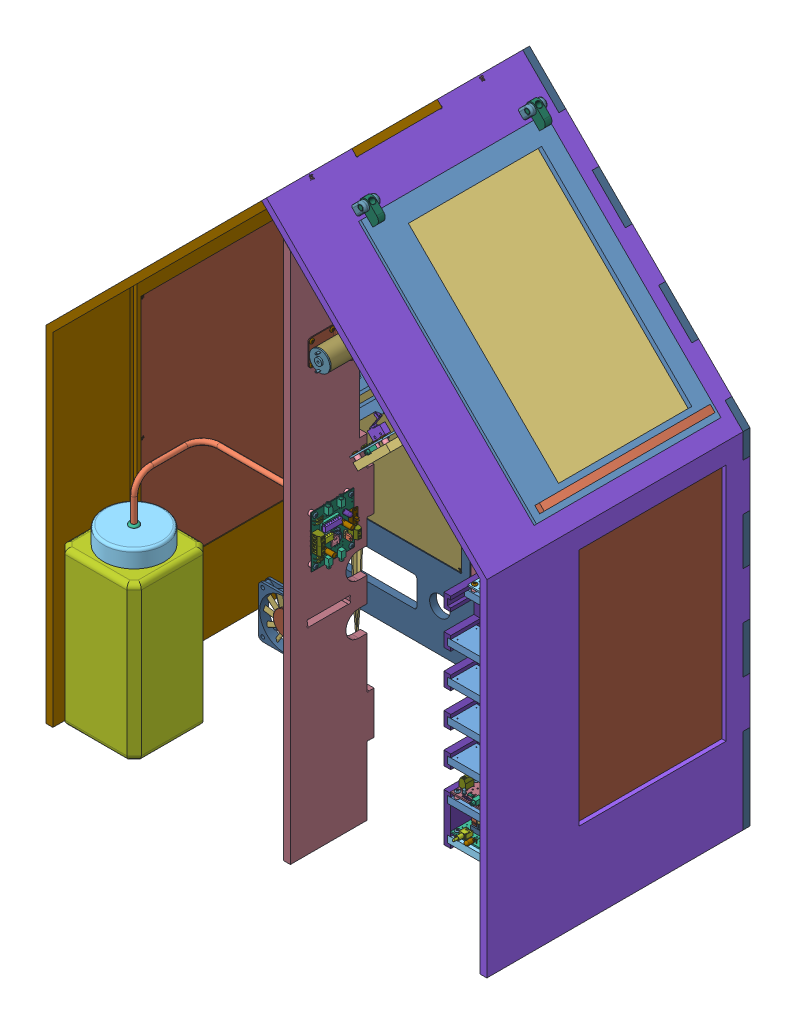
SolidWorks assembly Serre de base VDS, configuration guillotine. Lengths in mm.
Overall size (183.35 183.35 75.13).
351 component instances, 97 part files, 150 mates.
Components (placement in the parent):
- FONDINTERIEUR-1: FONDINTERIEUR [Défaut] at (-62.876 -300.5478 -4) (hidden)
- Crémallière M3-3-1: Crémallière M3-3 [Défaut] at (-39.5374 94.1308 4) x (0.707107 0.707107 0) z (0 0 1)
- Rondelle métal 3 x 12-1: Rondelle métal 3 x 12 [Défaut] at (57.939 191.6778 8)
- VIs TC 3 x 13-1: VIs TC 3 x 13 [Défaut] at (57.939 191.6778 2.4) x (1 0 0) z (0 -1 0) (hidden)
- VIs TC 3 x 13-2: VIs TC 3 x 13 [Défaut] at (22.5836 156.3225 2.4) x (1 0 0) z (0 -1 0) (hidden)
- Rondelle métal 3 x 12-2: Rondelle métal 3 x 12 [Défaut] at (22.5836 156.3225 8)
- Prépa 06 module Microrupteur-1: Prépa 06 module Microrupteur [Défaut] at (80.8247 148.8026 12.3834) x (0.707107 0.707107 0) z (-0.707107 0.707107 0) size (54 40.91 35.34)
  - support capteur-1: support capteur [Défaut] at (85.4284 22.7312 -4) size (54 38 8)
  - Entretoise CI-1: Entretoise CI [Défaut] at (-25.3985 -17.6166 4) size (5.9 5.9 4.1)
  - Entretoise CI-2: Entretoise CI [Défaut] at (-25.3985 4.3834 4) size (5.9 5.9 4.1)
  - Entretoise CI-3: Entretoise CI [Défaut] at (20.6015 -17.6166 4) size (5.9 5.9 4.1)
  - Entretoise CI-4: Entretoise CI [Défaut] at (20.6015 4.3834 4) size (5.9 5.9 4.1)
  - Module Microrupteur K-AP-MMR-1: Module Microrupteur K-AP-MMR [Défaut] at (24.602 -8.2581 10.6485) x (0 1 0) z (1 0 0) size (32.91 28.24 54)
    - CI-AP-MLBP avec jack-1: CI-AP-MLBP avec jack [Défaut] at (1.5279 -1.3102 0) size (32.91 8.01 54)
      - CI BP et DEL-1: CI BP et DEL [Défaut] at (-14.8869 -1.2382 0) size (30 1.6 54)
      - Embase jack 2.5-1: Embase jack 2.5 [Défaut] at (-14.8868 -1.2382 -27.0002) x (1 0 0) z (0 0 -1) size (10.81 8.01 5)
    - Résistance 10 K pas 11-1: Résistance 10 K pas 11 [Défaut] at (-6.8591 0.4515 -37.4997) x (0 0 -1) z (1 0 0) size (11.5 4.15 2.3)
    - Microrupteur-1: Microrupteur [Défaut] at (16.351 0.0515 -46.78) x (-1 0 0) z (0 0 -1) size (6.3 24.64 22.46)
  - VIs TC 3 x 6.5-1: VIs TC 3 x 6.5 [Défaut] at (-25.3985 -17.6166 3.3) x (1 0 0) z (0 -1 0) size (5.6 8.09 5.6)
  - VIs TC 3 x 6.5-2: VIs TC 3 x 6.5 [Défaut] at (-25.3979 4.3824 3.3) x (1 0 0) z (0 -1 0) size (5.6 8.09 5.6)
  - VIs TC 3 x 6.5-3: VIs TC 3 x 6.5 [Défaut] at (20.6015 -17.6166 3.3) x (0.418214 0.908348 0) z (0.908348 -0.418214 0) size (5.6 8.09 5.6)
  - VIs TC 3 x 6.5-4: VIs TC 3 x 6.5 [Défaut] at (20.6015 4.3834 3.3) x (1 0 0) z (0 -1 0) size (5.6 8.09 5.6)
- Prépa 06 module Microrupteur-2: Prépa 06 module Microrupteur [Défaut] at (10.114 78.0919 12.3834) x (0.707107 0.707107 0) z (-0.707107 0.707107 0) size (54 40.91 35.34)
  - support capteur-1: support capteur [Défaut] at (85.4284 22.7312 -4) size (54 38 8)
  - Entretoise CI-1: Entretoise CI [Défaut] at (-25.3985 -17.6166 4) size (5.9 5.9 4.1)
  - Entretoise CI-2: Entretoise CI [Défaut] at (-25.3985 4.3834 4) size (5.9 5.9 4.1)
  - Entretoise CI-3: Entretoise CI [Défaut] at (20.6015 -17.6166 4) size (5.9 5.9 4.1)
  - Entretoise CI-4: Entretoise CI [Défaut] at (20.6015 4.3834 4) size (5.9 5.9 4.1)
  - Module Microrupteur K-AP-MMR-1: Module Microrupteur K-AP-MMR [Défaut] at (24.602 -8.2581 10.6485) x (0 1 0) z (1 0 0) size (32.91 28.24 54)
    - CI-AP-MLBP avec jack-1: CI-AP-MLBP avec jack [Défaut] at (1.5279 -1.3102 0) size (32.91 8.01 54)
      - CI BP et DEL-1: CI BP et DEL [Défaut] at (-14.8869 -1.2382 0) size (30 1.6 54)
      - Embase jack 2.5-1: Embase jack 2.5 [Défaut] at (-14.8868 -1.2382 -27.0002) x (1 0 0) z (0 0 -1) size (10.81 8.01 5)
    - Résistance 10 K pas 11-1: Résistance 10 K pas 11 [Défaut] at (-6.8591 0.4515 -37.4997) x (0 0 -1) z (1 0 0) size (11.5 4.15 2.3)
    - Microrupteur-1: Microrupteur [Défaut] at (16.351 0.0515 -46.78) x (-1 0 0) z (0 0 -1) size (6.3 24.64 22.46)
  - VIs TC 3 x 6.5-1: VIs TC 3 x 6.5 [Défaut] at (-25.3985 -17.6166 3.3) x (1 0 0) z (0 -1 0) size (5.6 8.09 5.6)
  - VIs TC 3 x 6.5-2: VIs TC 3 x 6.5 [Défaut] at (-25.3979 4.3824 3.3) x (1 0 0) z (0 -1 0) size (5.6 8.09 5.6)
  - VIs TC 3 x 6.5-3: VIs TC 3 x 6.5 [Défaut] at (20.6015 -17.6166 3.3) x (0.418214 0.908348 0) z (0.908348 -0.418214 0) size (5.6 8.09 5.6)
  - VIs TC 3 x 6.5-4: VIs TC 3 x 6.5 [Défaut] at (20.6015 4.3834 3.3) x (1 0 0) z (0 -1 0) size (5.6 8.09 5.6)
- Ventilateur-1: Ventilateur [Défaut] at (-116.5864 -162.967 9.2) size (60 60 10.4)
  - Cage ventilateur-1: Cage ventilateur [Défaut] at (-27.2896 -30.9986 -5.2) size (60 60 10.4)
  - Hélice-1: Hélice [Défaut] at (3.0209 -0.9986 1.3) x (1 0 0) z (0 -1 0) size (55.32 5 55.41)
    - centre hélice-1: centre hélice [Défaut] at (-0.3105 -2.5 0) size (28.6 5 28.6)
    - Pale-1: Pale [Défaut] at (12.924 -1.982 -2.4379) x (-0.128403 0.431224 -0.893061) z (-0.06137 -0.902245 -0.426835) size (5.38 14.29 1.25)
    - Pale-12: Pale [Défaut] at (12.1411 -1.982 5.1043) x (0.374806 0.431224 -0.820711) z (0.179137 -0.902245 -0.392255) size (5.38 14.29 1.25)
    - Pale-13: Pale [Défaut] at (7.4049 -1.982 11.0258) x (0.759017 0.431224 -0.48779) z (0.362769 -0.902245 -0.233137) size (5.38 14.29 1.25)
    - Pale-14: Pale [Défaut] at (0.2191 -1.982 13.4468) x (0.902245 0.431224 0) z (0.431224 -0.902245 0) size (5.38 14.29 1.25)
    - Pale-15: Pale [Défaut] at (-7.1349 -1.982 11.5985) x (0.759017 0.431224 0.48779) z (0.362769 -0.902245 0.233137) size (5.38 14.29 1.25)
    - Pale-16: Pale [Défaut] at (-12.3221 -1.982 6.0677) x (0.374806 0.431224 0.820711) z (0.179137 -0.902245 0.392255) size (5.38 14.29 1.25)
    - Pale-17: Pale [Défaut] at (-13.6958 -1.982 -1.3895) x (-0.128403 0.431224 0.893061) z (-0.06137 -0.902245 0.426835) size (5.38 14.29 1.25)
    - Pale-18: Pale [Défaut] at (-10.8197 -1.982 -8.4055) x (-0.590845 0.431224 0.681871) z (-0.282392 -0.902245 0.325897) size (5.38 14.29 1.25)
    - Pale-19: Pale [Défaut] at (-4.6071 -1.982 -12.7529) x (-0.865698 0.431224 0.254192) z (-0.413756 -0.902245 0.12149) size (5.38 14.29 1.25)
    - Pale-20: Pale [Défaut] at (2.9697 -1.982 -13.0513) x (-0.865698 0.431224 -0.254192) z (-0.413756 -0.902245 -0.12149) size (5.38 14.29 1.25)
    - Pale-21: Pale [Défaut] at (9.505 -1.982 -9.206) x (-0.590845 0.431224 -0.681871) z (-0.282392 -0.902245 -0.325897) size (5.38 14.29 1.25)
- VIs TC 3 x 13-4: VIs TC 3 x 13 [Défaut] at (-138.876 -138.9656 8) x (1 0 0) z (0 -1 0) (hidden)
- VIs TC 3 x 13-6: VIs TC 3 x 13 [Défaut] at (-88.876 -138.9656 8) x (1 0 0) z (0 -1 0) (hidden)
- VIs TC 3 x 13-7: VIs TC 3 x 13 [Défaut] at (-88.876 -188.9656 8) x (1 0 0) z (0 -1 0) (hidden)
- VIs TC 3 x 13-8: VIs TC 3 x 13 [Défaut] at (-138.876 -188.9656 8) x (1 0 0) z (0 -1 0) (hidden)
- Entretoise CI-1: Entretoise CI [Défaut] at (57.939 191.6778 4) x (-0.97677 0.214292 0) z (0 0 1) size (5.9 5.9 4.1)
- Entretoise CI-2: Entretoise CI [Défaut] at (22.5836 156.3225 4) size (5.9 5.9 4.1)
- VIS TORCX TF 3 X 19-1: VIS TORCX TF 3 X 19 [Défaut] at (79.1287 147.1066 -4) x (-0.923728 -0.383049 0) z (0 0 -1) (hidden)
- VIS TORCX TF 3 X 19-2: VIS TORCX TF 3 X 19 [Défaut] at (8.418 76.3959 -4) x (-0.923728 -0.383049 0) z (0 0 -1) (hidden)
- Prépa 02 renfort arrière-1: Prépa 02 renfort arrière [Défaut] at (-30.876 -5.636 -123.7404) x (0 0 -1) z (1 0 0) size (98 630.07 61.8)
  - renfortarriere-1: renfortarriere [Défaut] at (-133.6202 -294.9118 -4) size (98 630.07 8)
  - Entretoise CI-1: Entretoise CI [Défaut] at (-194.2138 26.8323 4) size (5.9 5.9 4.1)
  - Entretoise CI-2: Entretoise CI [Défaut] at (-152.2157 27.0837 4) size (5.9 5.9 4.1)
  - Entretoise CI-3: Entretoise CI [Défaut] at (-193.9025 -25.1656 4) size (5.9 5.9 4.1)
  - Entretoise CI-4: Entretoise CI [Défaut] at (-151.9044 -24.9142 4) size (5.9 5.9 4.1)
  - VIs TC 3 x 9-1: VIs TC 3 x 9 [Défaut] at (-194.2138 26.8323 2.7) x (1 0 0) z (0 -1 0) size (5.6 10.69 5.6)
  - VIs TC 3 x 9-2: VIs TC 3 x 9 [Défaut] at (-152.2157 27.0837 2.7) x (1 0 0) z (0 -1 0) size (5.6 10.69 5.6)
  - VIs TC 3 x 9-3: VIs TC 3 x 9 [Défaut] at (-151.9044 -24.9142 2.7) x (1 0 0) z (0 -1 0) size (5.6 10.69 5.6)
  - VIs TC 3 x 9-4: VIs TC 3 x 9 [Défaut] at (-193.9025 -25.1656 2.7) x (1 0 0) z (0 -1 0) size (5.6 10.69 5.6)
  - Module 2 moteurs K-AP-MMOT-1: Module 2 moteurs K-AP-MMOT [Défaut] at (-148.0718 3.1444 10.7771) x (-0.005986 0.999982 0) z (0.999982 0.005986 0) size (65.82 19.5 50.56)
    - CI moteur-1: CI moteur [Défaut] at (-32.0357 -2.6771 0) size (60 1 50)
    - BORNIER 2-1: BORNIER 2 [Default] at (-17.0423 -1.6771 0.2294) x (0.999982 0 0.005986) z (0 1 0) size (9.97 7.55 15.02)
    - DEL D5 R-1: DEL D5 R [Défaut] at (9.6889 6.8229 -10.9906) x (1 0 0) z (0 -1 0) size (5.3 5.6 11.5)
    - Embase jack 2.5-1: Embase jack 2.5 [Défaut] at (-32.0356 -1.6771 -17.5006) size (10.81 8.01 5)
    - MICRO INVERSEUR A GLISSIERE-1: MICRO INVERSEUR A GLISSIERE [Défaut] at (3.55 3.3429 -4.0189) x (1 0 0.000537) z (0 1 0) size (19 5.82 12.15)
    - Résistance 220 ohm pas 11-1: Résistance 220 ohm pas 11 [Défaut] at (-10.0359 0.3229 -18.1991) x (-1 0 0) z (0 0 -1) size (11.5 4.15 2.3)
    - Embase jack 2.5-2: Embase jack 2.5 [Défaut] at (-32.0356 -1.6771 -32.5018) size (10.81 8.01 5)
    - Embase jack 2.5-3: Embase jack 2.5 [Défaut] at (27.964 -1.6771 -17.4981) x (-1 0 0) z (0 0 -1) size (10.81 8.01 5)
    - Embase jack 2.5-4: Embase jack 2.5 [Défaut] at (27.964 -1.6771 -32.4993) x (-1 0 0) z (0 0 -1) size (10.81 8.01 5)
    - Capuchon picot-1: Capuchon picot [Défaut] at (-16.1457 0.4729 -12.7155) x (1 0 0) z (0 -1 0) size (5.05 2.51 6.1)
    - ASB 3PICOTS-1: ASB 3PICOTS [Default] at (-9.9569 2.4259 -10.7946) x (1 0 0) z (0 -1 0) size (7.59 2.51 10)
      - PICOT-1: PICOT [Default] at (26.8516 -23.7306 1.953) size (2.51 2.51 10)
      - PICOT-2: PICOT [Default] at (29.3916 -23.7306 1.953) size (2.51 2.51 10)
      - PICOT-3: PICOT [Default] at (24.3116 -23.7306 1.953) size (2.51 2.51 10)
    - AJUSTABLE H-1: AJUSTABLE H [Défaut] at (-15.4716 0.3229 -24.988) x (0 0 1) z (0 1 0) size (8.6 10.76 7.4)
    - BORNIER 2-2: BORNIER 2 [Default] at (-2.0505 -1.6771 -50.2748) x (-1 0 0) z (0 1 0) size (9.97 7.55 15.02)
    - BORNIER 2-3: BORNIER 2 [Default] at (7.9495 -1.6771 -50.2748) x (-1 0 0) z (0 1 0) size (9.97 7.55 15.02)
    - Résistance 10 K pas 11-1: Résistance 10 K pas 11 [Défaut] at (19.1656 0.3229 -42.727) x (0 0 -1) z (1 0 0) size (11.5 4.15 2.3)
    - Résistance 10 K pas 11-2: Résistance 10 K pas 11 [Défaut] at (15.6274 0.3229 -42.6914) x (0 0 -1) z (1 0 0) size (11.5 4.15 2.3)
    - Résistance 10 K pas 11-3: Résistance 10 K pas 11 [Défaut] at (-19.5364 0.3229 -42.0005) x (0 0 -1) z (1 0 0) size (11.5 4.15 2.3)
    - Résistance 10 K pas 11-4: Résistance 10 K pas 11 [Défaut] at (-23.0365 0.3229 -42.0005) x (0 0 -1) z (1 0 0) size (11.5 4.15 2.3)
    - Support CI 8 pattes-1: Support CI 8 pattes [Défaut] at (-2.7368 -1.6771 -30.0083) x (0 0 -1) z (1 0 0) size (10 6 10.1)
    - Support CI 16 pattes-1: Support CI 16 pattes [Défaut] at (8.6068 -1.6771 -19.8458) x (0 0 -1) z (1 0 0) size (20.1 6 10.1)
    - CI 8 pattes-1: CI 8 pattes [Défaut] at (-2.7368 1.3229 -30.0113) x (0 0 -1) z (1 0 0) size (10 7.2 7.8)
    - CI 16 pattes-1: CI 16 pattes [Défaut] at (8.6068 1.3229 -19.8488) x (0 0 -1) z (1 0 0) size (20.1 7.2 7.8)
    - Capa 16V 100F 2.54-1: Capa 16V 100F 2.54 [Default] at (-14.0347 -26.6935 -37.5006) x (0 0 1) z (-1 0 0) size (5.2 15.5 5.88)
    - Capa 16V 100F 2.54-2: Capa 16V 100F 2.54 [Default] at (2.9618 -26.6935 -15.9995) x (0.999999 0 0.001464) z (-0.001464 0 0.999999) size (5.2 15.5 5.88)
    - condensateur 100nF-1: condensateur 100nF [Default] at (-2.9304 -7.4359 -15.4031) x (0 0 -1) z (1 0 0) size (5.85 10.35 1.99)
    - condensateur 100nF-2: condensateur 100nF [Default] at (0.5738 -7.4359 -15.3738) x (0 0 -1) z (1 0 0) size (5.85 10.35 1.99)
  - Moteur MFA 12-24V-1: Moteur MFA 12-24V [Défaut] at (-181.5572 189.3895 16.5047) x (-1 0 0) z (0 1 0) size (70.4 27.9 30)
    - Support moteur-1: Support moteur [Défaut] at (-14.3868 -12.5047 0) size (31 26.4 30)
    - Corps moteur-1: Corps moteur [Défaut] at (14.8132 1.8953 0) x (0 0 1) z (-1 0 0) size (24 24 63.9)
    - Capuchon moteur-1: Capuchon moteur [Défaut] at (-15.3868 1.8953 0) x (0 0 1) z (-1 0 0) size (27 27 18.7)
    - Arrière moteur-1: Arrière moteur [Défaut] at (16.3132 1.8953 0) x (0 0 1) z (-1 0 0) size (24 24 6.5)
  - Prépa 01 roue dentée-1: Prépa 01 roue dentée [Défaut] at (-131.9704 192.8178 10.3013) x (0 0.156764 -0.987636) z (1 0 0) size (54 54 14)
    - roue dentée 16-1: roue dentée 16 [Défaut] at (-7.1573 -1.556 -4) size (54 54 8)
    - Bague d'arrêt 4x12x24-1: Bague d'arrêt 4x12x24 [Défaut] at (-8.536 -2.1164 -10) x (0 1 0) z (0 0 1) size (24 24 8)
    - VIs TC 3 x 6.5-1: VIs TC 3 x 6.5 [Défaut] at (-8.536 6.8836 2.4) x (1 0 0) z (0 1 0) size (5.6 8.09 5.6)
    - VIs TC 3 x 6.5-2: VIs TC 3 x 6.5 [Défaut] at (-8.536 -11.1164 2.4) x (1 0 0) z (0 1 0) size (5.6 8.09 5.6)
  - VIs TC 3 x 6.5-1: VIs TC 3 x 6.5 [Défaut] at (-194.1704 201.3895 -1.4) x (1 0 0) z (0 -1 0) size (5.6 8.09 5.6)
  - VIs TC 3 x 6.5-2: VIs TC 3 x 6.5 [Défaut] at (-170.1704 201.3895 -1.4) x (1 0 0) z (0 -1 0) size (5.6 8.09 5.6)
  - VIs TC 3 x 6.5-3: VIs TC 3 x 6.5 [Défaut] at (-194.1704 177.3895 -1.4) x (1 0 0) z (0 -1 0) size (5.6 8.09 5.6)
  - VIs TC 3 x 6.5-4: VIs TC 3 x 6.5 [Défaut] at (-170.1704 177.3895 -1.4) x (1 0 0) z (0 -1 0) size (5.6 8.09 5.6)
- étagèrebrumi-1: étagèrebrumi [Défaut] at (-62.876 -93.9656 245.3364) x (1 0 0) z (0 1 0) (hidden)
- VIS TORCX TF 3 X 19-3: VIS TORCX TF 3 X 19 [Défaut] at (-30.876 -315.9656 -4) x (-0.991079 -0.133274 0) z (0 0 -1) (hidden)
- VIS TORCX TF 3 X 19-4: VIS TORCX TF 3 X 19 [Défaut] at (-30.876 -274.5499 -4) x (-0.991079 -0.133274 0) z (0 0 -1) (hidden)
- VIS TORCX TF 3 X 19-5: VIS TORCX TF 3 X 19 [Défaut] at (-169.876 -89.9656 -4) x (-0.991079 -0.133274 0) z (0 0 -1) (hidden)
- VIS TORCX TF 3 X 19-6: VIS TORCX TF 3 X 19 [Défaut] at (-30.876 -27.0369 -4) x (-0.991079 -0.133274 0) z (0 0 -1) (hidden)
- VIS TORCX TF 3 X 19-7: VIS TORCX TF 3 X 19 [Défaut] at (-30.876 278.5344 -4) x (-0.991079 -0.133274 0) z (0 0 -1) (hidden)
- Coté gauche serre-1: Coté gauche serre [Défaut] at (-304.876 -288.0405 43.9648) x (0 0 -1) z (1 0 0) (hidden)
- Coté support brumisateur-1: Coté support brumisateur [Défaut] at (-87.876 -76.5368 52.2063) x (0 0 1) z (-1 0 0) (hidden)
- Coté support brumisateur-2: Coté support brumisateur [Défaut] at (-204.876 -76.5368 52.2063) x (0 0 1) z (-1 0 0) (hidden)
- Renfort bidon-1: Renfort bidon [Défaut] at (-206.376 -195.9656 85) x (1 0 0) z (0 1 0) (hidden)
- suportbloceau-1: suportbloceau [Défaut] at (-238.3888 -323.9656 72.4161) x (1 0 0) z (0 1 0) (hidden)
- VIS TORCX TF 3 X 19-12: VIS TORCX TF 3 X 19 [Défaut] at (-198.876 -191.9656 -4) x (-0.923728 -0.383049 0) z (0 0 -1) (hidden)
- VIS TORCX TF 3 X 19-13: VIS TORCX TF 3 X 19 [Défaut] at (-164.4919 -191.9656 -4) x (-0.923728 -0.383049 0) z (0 0 -1) (hidden)
- VIS TORCX TF 3 X 19-14: VIS TORCX TF 3 X 19 [Défaut] at (-208.876 -75.9656 -4) x (-0.923728 -0.383049 0) z (0 0 -1) (hidden)
- VIS TORCX TF 3 X 19-15: VIS TORCX TF 3 X 19 [Défaut] at (-208.876 -16.4656 -4) x (-0.923728 -0.383049 0) z (0 0 -1) (hidden)
- VIS TORCX TF 3 X 19-16: VIS TORCX TF 3 X 19 [Défaut] at (-91.876 -75.9656 -4) x (-0.923728 -0.383049 0) z (0 0 -1) (hidden)
- VIS TORCX TF 3 X 19-17: VIS TORCX TF 3 X 19 [Défaut] at (-91.876 -15.9656 -4) x (-0.923728 -0.383049 0) z (0 0 -1) (hidden)
- VIS TORCX TF 3 X 19-18: VIS TORCX TF 3 X 19 [Défaut] at (-304.876 -89.9656 48.9996) x (0 0 1) z (-1 0 0) (hidden)
- VIS TORCX TF 3 X 19-25: VIS TORCX TF 3 X 19 [Défaut] at (-304.876 -248.9656 -0.0009) x (0 0 1) z (-1 0 0) (hidden)
- VIS TORCX TF 3 X 19-26: VIS TORCX TF 3 X 19 [Défaut] at (-300.876 -323.9656 49) x (0.782535 0 -0.622606) z (0 -1 0) (hidden)
- VIS TORCX TF 3 X 19-29: VIS TORCX TF 3 X 19 [Défaut] at (-271.876 -323.9656 0) x (0.782535 0 -0.622606) z (0 -1 0) (hidden)
- VIS TORCX TF 3 X 19-30: VIS TORCX TF 3 X 19 [Défaut] at (-179.876 -323.9656 0) x (0.782535 0 -0.622606) z (0 -1 0) (hidden)
- Coté droit serre-1: Coté droit serre [Défaut] at (187.124 -288.4466 43.9657) x (0 0 -1) z (1 0 0) (hidden)
- VIS TORCX TF 3 X 19-35: VIS TORCX TF 3 X 19 [Défaut] at (195.124 -248.9656 0) x (0 -0.192039 -0.981387) z (1 0 0) (hidden)
- Poutre fond-1: Poutre fond [Défaut] at (-62.876 -231.9656 64.5822) x (1 0 0) z (0 1 0) (hidden)
- VIS TORCX TF 3 X 19-36: VIS TORCX TF 3 X 19 [Défaut] at (-213.1345 -227.9656 4) (hidden)
- VIS TORCX TF 3 X 19-37: VIS TORCX TF 3 X 19 [Défaut] at (-54.876 -227.9656 4) (hidden)
- Poutre plateau-1: Poutre plateau [Défaut] at (79.7388 -229.6404 -13) x (-1 0 0) z (0 0 -1) (hidden)
- façadeporteplateau-1: façadeporteplateau [Défaut] at (102.5126 -276.3164 -206) (hidden)
- VIS TORCX TF 3 X 19-38: VIS TORCX TF 3 X 19 [Défaut] at (191.124 -273.9656 -206) x (-0.923728 -0.383049 0) z (0 0 -1) (hidden)
- VIS TORCX TF 3 X 19-39: VIS TORCX TF 3 X 19 [Défaut] at (195.124 -308.9656 -202) x (0 0 -1) z (1 0 0) (hidden)
- VIS TORCX TF 3 X 19-40: VIS TORCX TF 3 X 19 [Défaut] at (195.124 -238.9656 -202) x (0 0 -1) z (1 0 0) (hidden)
- VIS TORCX TF 3 X 19-43: VIS TORCX TF 3 X 19 [Défaut] at (-300.876 -273.9656 -206) x (-0.923728 -0.383049 0) z (0 0 -1) (hidden)
- VIS TORCX TF 3 X 19-44: VIS TORCX TF 3 X 19 [Défaut] at (-304.876 -238.9737 -202) x (0 0 1) z (-1 0 0) (hidden)
- VIS TORCX TF 3 X 19-45: VIS TORCX TF 3 X 19 [Défaut] at (-304.876 -308.9656 -202) x (0 0 1) z (-1 0 0) (hidden)
- VIS TORCX TF 3 X 19-49: VIS TORCX TF 3 X 19 [Défaut] at (103.3825 -227.9656 4) (hidden)
- Sous ensemble Rack module-1: Sous ensemble Rack module [Défaut] at (116.8547 -126.3174 -67.6389) x (0 0 -1) z (1 0 0) size (70.07 263.1 323.21)
  - rack coté gauche-1: rack coté gauche [Défaut] at (-102.2159 -95.6801 -4) size (58 256 8)
  - rack coté droit-1: rack coté droit [Défaut] at (-102.2159 -95.6628 58) size (58 256 8)
  - Prépa 05 module TEMP-1: Prépa 05 module TEMP [Défaut] at (-82.7846 122.513 33.0896) x (0 0 1) z (0 1 0) size (62 41.41 19.08)
    - supportcarterack-1: supportcarterack [Défaut] at (3.5074 9.0286 -6.1612) size (62 30 8)
    - Entretoise CI-1: Entretoise CI [Défaut] at (-25.0896 -14.8542 1.8388) size (5.9 5.9 4.1)
    - Entretoise CI-2: Entretoise CI [Défaut] at (-25.0896 7.1458 1.8388) size (5.9 5.9 4.1)
    - Entretoise CI-3: Entretoise CI [Défaut] at (20.9104 -14.8542 1.8388) size (5.9 5.9 4.1)
    - Entretoise CI-4: Entretoise CI [Défaut] at (20.9104 7.1458 1.8388) size (5.9 5.9 4.1)
    - Module temperature K-AP-MTEMP-1: Module temperature K-AP-MTEMP [Défaut] at (24.9109 -3.9678 7.1771) x (0 1 0) z (1 0 0) size (41.41 8.39 54)
      - CI BP et DEL-1: CI BP et DEL [Défaut] at (-14.8869 -1.2382 0) size (30 1.6 54)
      - Embase jack 2.5-1: Embase jack 2.5 [Défaut] at (-14.8868 0.3618 -27.0002) size (10.81 8.01 5)
      - Résistance 3,9 K pas 11-1: Résistance 3,9 K pas 11 [Défaut] at (-12.3875 1.7618 -37.4997) x (0 0 1) z (-1 0 0) size (11.5 4.15 2.3)
      - RC1 Tansistor plié 90°-1: RC1 Tansistor plié 90° [Défaut] at (18.6119 3.3399 -22.4989) x (0 0 -1) z (0 -1 0) size (4.8 10.25 6.98)
    - VIs TC 3 x 6.5-1: VIs TC 3 x 6.5 [Défaut] at (-25.0896 -14.8542 1.1388) x (1 0 0) z (0 -1 0) size (5.6 8.09 5.6)
    - VIs TC 3 x 6.5-2: VIs TC 3 x 6.5 [Défaut] at (-25.0896 7.1458 1.1388) x (1 0 0) z (0 -1 0) size (5.6 8.09 5.6)
    - VIs TC 3 x 6.5-3: VIs TC 3 x 6.5 [Défaut] at (20.9104 7.1458 1.1388) x (1 0 0) z (0 -1 0) size (5.6 8.09 5.6)
    - VIs TC 3 x 6.5-4: VIs TC 3 x 6.5 [Défaut] at (20.9104 -14.8542 1.1388) x (1 0 0) z (0 -1 0) size (5.6 8.09 5.6)
  - VIS TORCX TF 3 X 19-1: VIS TORCX TF 3 X 19 [Défaut] at (-86.6389 120.3518 66)
  - VIS TORCX TF 3 X 19-2: VIS TORCX TF 3 X 19 [Défaut] at (-86.6389 120.3431 -4) x (-0.923728 -0.383049 0) z (0 0 -1)
  - Prépa 04 module MAFU-1: Prépa 04 module MAFU [Défaut] at (-94.8752 -119.6656 28.2245) x (0 0 1) z (0 1 0) size (62 61.57 27.12)
    - basesuportpuissance-1: basesuportpuissance [Défaut] at (-4.8343 -1.5394 -4) size (62 50 8)
    - Entretoise CI-1: Entretoise CI [Défaut] at (-20.2245 -22.7636 4) size (5.9 5.9 4.1)
    - Entretoise CI-2: Entretoise CI [Défaut] at (-20.2245 -0.7636 4) size (5.9 5.9 4.1)
    - Entretoise CI-3: Entretoise CI [Défaut] at (25.7755 -0.7636 4) size (5.9 5.9 4.1)
    - Entretoise CI-4: Entretoise CI [Défaut] at (25.7755 -22.7636 4) size (5.9 5.9 4.1)
    - CI-MAFU avec borniers-1: CI-MAFU avec borniers [Défaut] at (2.9088 -18.7288 8.9) x (0 -1 0) z (0 0 1) size (43.65 54 18.42)
      - CI-MAFU-1: CI-MAFU [Défaut] at (-21.9652 -27.1333 -0.8) size (30 54 1.6)
      - Inter long à souder 734-7220-1: Inter long à souder 734-7220 [Défaut] at (8.1051 -9.1203 1.3) x (-1 0 0) z (0 1 0) size (20.8 9.2 8)
      - Embase femelle d'alimentation-1: Embase femelle d'alimentation [Défaut] at (4.7338 12.8853 0.8) x (0 -1 0) z (-1 0 0) size (10.39 15 14.1)
      - DEL D5 rouge pliée-2: DEL D5 rouge pliée [Défaut] at (17.5325 -1.131 5.2) x (0 1 0) z (-1 0 0) size (5.3 8.8 12.9)
      - Support fusible avec fusible-1: Support fusible avec fusible [Défaut] at (-8.3615 -5.1853 4.8987) x (0 1 0) z (1 0 0) size (23 17 8.6)
        - Support fusible base-1: Support fusible base [Défaut] at (-10.9359 -4.0987 -4.3) size (22 7 8.6)
        - Support fusible contact-1: Support fusible contact [Défaut] at (5.4641 0.8731 -0.0014) size (6.1 17 6.2)
        - Support fusible contact-2: Support fusible contact [Défaut] at (-5.3359 0.8731 -0.0014) x (-1 0 0) z (0 0 -1) size (6.1 17 6.2)
        - Fusible-1: Fusible [Défaut] at (-0.0359 6.2731 -0.0014) size (19.8 5.2 5.2)
      - BORNIER 2-2: BORNIER 2 [Default] at (-24.0402 -10.1483 0.8) x (0 -1 0) z (0 0 1) size (9.97 7.55 15.02)
      - BORNIER 2-4: BORNIER 2 [Default] at (-24.0402 -0.1483 0.8) x (0 -1 0) z (0 0 1) size (9.97 7.55 15.02)
      - BORNIER 2-5: BORNIER 2 [Default] at (-24.0402 9.8517 0.8) x (0 -1 0) z (0 0 1) size (9.97 7.55 15.02)
      - BORNIER 2-6: BORNIER 2 [Default] at (-24.0402 19.8517 0.8) x (0 -1 0) z (0 0 1) size (9.97 7.55 15.02)
    - VIs TC 3 x 9-1: VIs TC 3 x 9 [Défaut] at (-20.2245 -22.7636 3.3) x (1 0 0) z (0 -1 0) size (5.6 10.69 5.6)
    - VIs TC 3 x 9-2: VIs TC 3 x 9 [Défaut] at (25.7755 -22.7636 3.3) x (1 0 0) z (0 -1 0) size (5.6 10.69 5.6)
    - VIs TC 3 x 9-3: VIs TC 3 x 9 [Défaut] at (-20.2245 -0.7636 3.3) x (1 0 0) z (0 -1 0) size (5.6 10.69 5.6)
    - VIs TC 3 x 9-4: VIs TC 3 x 9 [Défaut] at (25.7755 -0.7636 3.3) x (1 0 0) z (0 -1 0) size (5.6 10.69 5.6)
  - VIS TORCX TF 3 X 19-3: VIS TORCX TF 3 X 19 [Défaut] at (-107.1389 -119.6824 66)
  - VIS TORCX TF 3 X 19-4: VIS TORCX TF 3 X 19 [Défaut] at (-78.1389 -119.6824 66)
  - VIS TORCX TF 3 X 19-6: VIS TORCX TF 3 X 19 [Défaut] at (-107.1389 -119.6656 -4) x (-0.923728 -0.383049 0) z (0 0 -1)
  - VIS TORCX TF 3 X 19-7: VIS TORCX TF 3 X 19 [Défaut] at (-78.1389 -119.6656 -4) x (-0.923728 -0.383049 0) z (0 0 -1)
  - Prépa 03 module PWR-1: Prépa 03 module PWR [Défaut] at (-104.636 -79.6656 32.1892) x (0 0 1) z (0 1 0) size (62 33.06 23.72)
    - supportcarterack-1: supportcarterack [Défaut] at (4.4079 10.88 -4) size (62 30 8)
    - Entretoise CI-1: Entretoise CI [Défaut] at (-24.1892 -13.0028 4) size (5.9 5.9 4.1)
    - Entretoise CI-2: Entretoise CI [Défaut] at (-24.1892 8.9972 4) size (5.9 5.9 4.1)
    - Entretoise CI-3: Entretoise CI [Défaut] at (21.8108 8.9972 4) size (5.9 5.9 4.1)
    - Entretoise CI-4: Entretoise CI [Défaut] at (21.8108 -13.0028 4) size (5.9 5.9 4.1)
    - Module K-AP-MPWR-1: Module K-AP-MPWR [Défaut] at (-1.2571 1.9363 8.9) x (0 1 0) z (0 0 1) size (33.06 54.47 15.02)
      - CI AP-PWR-1: CI AP-PWR [Défaut] at (-18.9391 -27.0679 -0.8) size (30 54 1.6)
      - BORNIER 2-1: BORNIER 2 [Default] at (0.963 27.1235 0.8) x (-1 0 0) z (0 0 1) size (9.97 7.55 15.02)
      - DELverte 3mm-1: DELverte 3mm [Défaut] at (-12.9358 16.93 1.8) x (0 0 1) z (-1 0 0) size (7.4 3.42 3.8)
      - diode-1: diode [Défaut] at (-12.9396 11.4315 3.2) x (1 0 0) z (0 -1 0) size (2.65 5.32 8.12)
      - ASB 3PICOTS avec capuchon-1: ASB 3PICOTS avec capuchon [Default] at (-16.084 -16.9024 4.903) x (-1 0 0) z (0 0 -1) size (7.59 2.51 10.25)
        - PICOT-1: PICOT [Default] at (26.8516 -23.7306 1.953) size (2.51 2.51 10)
        - PICOT-2: PICOT [Default] at (29.3916 -23.7306 1.953) size (2.51 2.51 10)
        - PICOT-3: PICOT [Default] at (24.3116 -23.7306 1.953) size (2.51 2.51 10)
        - Capuchon picot-1: Capuchon picot [Défaut] at (-6.1888 -1.9209 1.953) size (5.05 2.51 6.1)
      - Embase jack 2.5-1: Embase jack 2.5 [Défaut] at (-18.9403 -0.0677 0.8) x (1 0 0) z (0 -1 0) size (10.81 8.01 5)
      - REG-1: REG [Default] at (-4.2884 5.0073 0.8) x (0 -1 0) z (0 0 1) size (10.15 20.05 5.19)
      - Résistance 220 pas 11-1: Résistance 220 pas 11 [Défaut] at (-17.2386 9.3312 2.2) x (0 -1 0) z (-1 0 0) size (11.5 4.15 2.3)
      - Résistance 10K pas de 11-1: Résistance 10K pas de 11 [Défaut] at (-17.2386 -9.3683 2.2) x (0 -1 0) z (-1 0 0) size (11.5 4.15 2.3)
      - BORNIER 2-2: BORNIER 2 [Default] at (-8.9238 -27.3428 0.8) size (9.97 7.55 15.02)
    - VIs TC 3 x 9-1: VIs TC 3 x 9 [Défaut] at (-24.1892 -13.0028 3.3) x (1 0 0) z (0 -1 0) size (5.6 10.69 5.6)
    - VIs TC 3 x 9-2: VIs TC 3 x 9 [Défaut] at (-24.1892 8.9972 3.3) x (1 0 0) z (0 -1 0) size (5.6 10.69 5.6)
    - VIs TC 3 x 9-3: VIs TC 3 x 9 [Défaut] at (21.8108 8.9972 3.3) x (1 0 0) z (0 -1 0) size (5.6 10.69 5.6)
    - VIs TC 3 x 9-4: VIs TC 3 x 9 [Défaut] at (21.8108 -13.0028 3.3) x (1 0 0) z (0 -1 0) size (5.6 10.69 5.6)
  - supportcarterack-1: supportcarterack [Défaut] at (-119.5217 -35.6656 36.597) x (0 0 1) z (0 -1 0) size (62 30 8)
  - supportcarterack-2: supportcarterack [Défaut] at (-119.5217 4.3344 36.597) x (0 0 1) z (0 -1 0) size (62 30 8)
  - supportcarterack-3: supportcarterack [Défaut] at (-119.5217 44.3344 36.597) x (0 0 1) z (0 -1 0) size (62 30 8)
  - supportcarterack-4: supportcarterack [Défaut] at (-119.5217 84.3344 36.597) x (0 0 1) z (0 -1 0) size (62 30 8)
- VIS TORCX TF 3 X 19-50: VIS TORCX TF 3 X 19 [Défaut] at (178.8547 -145.9656 -4) x (-0.923728 -0.383049 0) z (0 0 -1) (hidden)
- VIS TORCX TF 3 X 19-51: VIS TORCX TF 3 X 19 [Défaut] at (116.8547 -145.9656 -4) x (-0.923728 -0.383049 0) z (0 0 -1) (hidden)
- VIS TORCX TF 3 X 19-52: VIS TORCX TF 3 X 19 [Défaut] at (178.8547 -7.9656 -4) x (-0.923728 -0.383049 0) z (0 0 -1) (hidden)
- VIS TORCX TF 3 X 19-53: VIS TORCX TF 3 X 19 [Défaut] at (116.8547 -7.9656 -4) x (-0.923728 -0.383049 0) z (0 0 -1) (hidden)
- Sous ensemble Arrosage-1: Sous ensemble Arrosage [Défaut] at (-248.1801 -261.6655 37.8651) x (-0.00308 0 0.999995) z (0 -1 0) size (140.54 240.54 274.35)
  - Pompe-1: Pompe [Défaut] at (-9.0938 -0.5877 17.5) size (40 29 55)
  - Tuyau gouteur-1: Tuyau gouteur [Défaut] at (-69.6171 -162.8404 -195.5) x (0 0 -1) z (0.999995 -0.00308 0) size (203 173 86)
  - Gouteur-1: Gouteur [Défaut] at (-70.8858 -170.9803 -151.85) x (-0.999995 0.00308 0) z (0 0 1) size (21 26.3 133.2)
    - PiedGouteur-1: PiedGouteur [Défaut] at (-1.2437 2.6563 -65) size (16 23.8 130)
    - BouchonGouteur-1: BouchonGouteur [Défaut] at (-1.2437 2.6563 -57) x (-0.923728 -0.383049 0) z (0 0 -1) size (16.07 16.07 11.2)
  - Bouchon reservoir-1: Bouchon reservoir [Défaut] at (10.9062 6.9123 -125.7) x (0.574699 -0.818365 0) z (0.818365 0.574699 0) size (71 20 71)
  - Passe cable-1: Passe cable [Défaut] at (10.9062 6.9123 -169.9434) x (0 0 -1) z (0 1 0) size (6 11 11)
  - Reservoir 1,25L-1: Reservoir 1,25L [Défaut] at (7.3532 24.2973 -125.7) x (0.999995 -0.00308 0) z (0 0 1) size (89.5 89.5 187)
- plateau base-1: plateau base [Défaut] at (-230.7684 -235.9656 -41.3241) x (1 0 0) z (0 1 0) (hidden)
- fondcuivré-1: fondcuivré [Défaut] at (-208.3657 -251.1382 -5) (hidden)
- Capot complet-1: Capot complet [Vitres] at (-187.0166 -15.8593 -60) x (-1 0 0) z (0 0 -1) size (516 661.85 308)
  - Capot coté droit-1: Capot coté droit [Défaut] at (-332.1697 -265.6526 -154) size (263.66 661.85 308)
  - Capot coté gauche-1: Capot coté gauche [Défaut] at (175.8303 -266.1888 -154) size (263.66 661.85 308)
  - Capotfaçade-1: Capotfaçade [Défaut] at (75.9652 -264.3201 154) x (-1 0 0) z (0 0 -1) size (516 661.85 8)
  - Vitre laterale-1: Vitre laterale [Défaut] at (-385.1406 -165.6883 102.4285) x (0 1 0) z (1 0 0) size (290.43 181.9 2)
  - Vitre avant grande-1: Vitre avant grande [Défaut] at (-355.6546 -169.3327 147) x (0 1 0) z (0 0 1) size (286.8 171.11 2)
  - Vitre laterale-2: Vitre laterale [Défaut] at (120.8594 30.4421 102.4285) x (0 -1 0) z (-1 0 0) size (290.43 181.9 2)
  - Vitre avant grande-2: Vitre avant grande [Défaut] at (-40.8684 -169.3327 147) x (0 1 0) z (0 0 1) size (286.8 171.11 2)
  - Vitre avant centrale-1: Vitre avant centrale [Défaut] at (-154.2178 43.2096 147) size (123.47 286.8 2)
  - Vitre laterale-4: Vitre laterale [Défaut] at (-65.085 276.7887 -22.3285) x (0.707107 -0.707107 0) z (0.707107 0.707107 0) size (290.43 181.9 2)
  - Charnière percée-1: Charnière percée [Défaut] at (-176.8635 321.0541 -74.2825) x (-0.707107 -0.707107 0) z (0 0 -1) size (25.5 17 19)
    - Charnière percée-1: Charnière percée [Défaut] at (-8.739 -12.0088 -9.5) size (11 16 19)
    - Charnièere percée  2-1: Charnièere percée  2 [Défaut] at (-8.739 1.9912 -4) size (25.5 13 19)
  - Charnière percée-2: Charnière percée [Défaut] at (-176.8635 321.0541 120.9123) x (-0.707107 -0.707107 0) z (0 0 -1) size (25.5 17 19)
    - Charnière percée-1: Charnière percée [Défaut] at (-8.739 -12.0088 -9.5) size (11 16 19)
    - Charnièere percée  2-1: Charnièere percée  2 [Défaut] at (-8.739 1.9912 -4) size (25.5 13 19)
  - VIS TORCX TF 3 X 13-4: VIS TORCX TF 3 X 13 [Défaut] at (-159.0106 315.56 -74.2825) x (0.5 0.5 -0.707107) z (0.707107 -0.707107 0) size (5.6 5.6 13)
  - VIS TORCX TF 3 X 13-5: VIS TORCX TF 3 X 13 [Défaut] at (-159.0106 315.56 120.9123) x (0.5 0.5 -0.707107) z (0.707107 -0.707107 0) size (5.6 5.6 13)
  - VIS TORCX TF 3 X 19-1: VIS TORCX TF 3 X 19 [Défaut] at (-386.1406 -283.1062 154)
  - VIS TORCX TF 3 X 19-2: VIS TORCX TF 3 X 19 [Défaut] at (-386.1406 -233.1062 154)
  - VIS TORCX TF 3 X 19-3: VIS TORCX TF 3 X 19 [Défaut] at (-386.1406 -125.6062 154)
  - VIS TORCX TF 3 X 19-4: VIS TORCX TF 3 X 19 [Défaut] at (-386.1406 -15.6062 154)
  - VIS TORCX TF 3 X 19-5: VIS TORCX TF 3 X 19 [Défaut] at (-386.1406 81.3179 154)
  - VIS TORCX TF 3 X 19-6: VIS TORCX TF 3 X 19 [Défaut] at (-376.7525 103.4731 154)
  - VIS TORCX TF 3 X 19-7: VIS TORCX TF 3 X 19 [Défaut] at (-307.8566 172.3691 154)
  - VIS TORCX TF 3 X 19-8: VIS TORCX TF 3 X 19 [Défaut] at (-230.0748 250.1508 154)
  - VIS TORCX TF 3 X 19-9: VIS TORCX TF 3 X 19 [Défaut] at (-150.5253 329.7003 154)
  - VIS TORCX TF 3 X 19-10: VIS TORCX TF 3 X 19 [Défaut] at (-134.969 350.9153 96) x (0.5 0.5 0.707107) z (-0.707107 0.707107 0)
  - VIS TORCX TF 3 X 19-11: VIS TORCX TF 3 X 19 [Défaut] at (-129.3121 350.9153 -4) x (0.5 -0.5 -0.707107) z (0.707107 0.707107 0)
  - VIS TORCX TF 3 X 19-22: VIS TORCX TF 3 X 19 [Défaut] at (-134.969 350.9153 -104) x (0.5 0.5 0.707107) z (-0.707107 0.707107 0)
  - VIS TORCX TF 3 X 19-24: VIS TORCX TF 3 X 19 [Défaut] at (-113.7558 329.7003 154)
  - VIS TORCX TF 3 X 19-25: VIS TORCX TF 3 X 19 [Défaut] at (-34.2063 250.1508 154)
  - VIS TORCX TF 3 X 19-26: VIS TORCX TF 3 X 19 [Défaut] at (43.5755 172.3691 154)
  - VIS TORCX TF 3 X 19-27: VIS TORCX TF 3 X 19 [Défaut] at (112.4714 103.4731 154)
  - VIS TORCX TF 3 X 19-28: VIS TORCX TF 3 X 19 [Défaut] at (121.8594 81.3179 154)
  - VIS TORCX TF 3 X 19-29: VIS TORCX TF 3 X 19 [Défaut] at (121.8594 -15.6062 154)
  - VIS TORCX TF 3 X 19-30: VIS TORCX TF 3 X 19 [Défaut] at (121.8594 -233.1062 154)
  - VIS TORCX TF 3 X 19-31: VIS TORCX TF 3 X 19 [Défaut] at (121.8594 -125.6062 154)
  - VIS TORCX TF 3 X 19-32: VIS TORCX TF 3 X 19 [Défaut] at (121.8594 -283.1062 154)
  - Aimant-1: Aimant [Défaut] at (122.8594 -288.1062 -134) x (0 0 1) z (-1 0 0) size (8 8 5)
  - Aimant-2: Aimant [Défaut] at (-387.1406 -288.1062 -134) x (0 0 -1) z (1 0 0) size (8 8 5)
  - VIS TF 2.2x6.4-114: VIS TF 2.2x6.4 [Défaut] at (-383.1406 75.3601 128.5) x (0 -1 0) z (1 0 0) size (4.2 4.2 6.4)
  - VIS TF 2.2x6.4-115: VIS TF 2.2x6.4 [Défaut] at (-383.1406 -67.3599 128.5) x (0 -1 0) z (1 0 0) size (4.2 4.2 6.4)
  - VIS TF 2.2x6.4-116: VIS TF 2.2x6.4 [Défaut] at (-383.1406 -210.0699 128.5) x (0 -1 0) z (1 0 0) size (4.2 4.2 6.4)
  - VIS TF 2.2x6.4-117: VIS TF 2.2x6.4 [Défaut] at (-383.2825 -210.0699 -48.4) x (0 -1 0) z (0 0 1) size (4.2 4.2 6.4)
  - VIS TF 2.2x6.4-118: VIS TF 2.2x6.4 [Défaut] at (-383.2825 -67.3599 -48.4) x (0 -1 0) z (0 0 1) size (4.2 4.2 6.4)
  - VIS TF 2.2x6.4-119: VIS TF 2.2x6.4 [Défaut] at (-383.2825 75.3601 -48.4) x (0 -1 0) z (0 0 1) size (4.2 4.2 6.4)
  - VIS TF 2.2x6.4-120: VIS TF 2.2x6.4 [Défaut] at (-372.6406 -210.6062 147) x (1 0 0) z (0 0 -1) size (4.2 4.2 6.4)
  - VIS TF 2.2x6.4-121: VIS TF 2.2x6.4 [Défaut] at (-206.5306 -210.6062 147) x (1 0 0) z (0 0 -1) size (4.2 4.2 6.4)
  - VIS TF 2.2x6.4-122: VIS TF 2.2x6.4 [Défaut] at (-191.4267 -210.6062 147) x (1 0 0) z (0 0 -1) size (4.2 4.2 6.4)
  - VIS TF 2.2x6.4-123: VIS TF 2.2x6.4 [Défaut] at (-72.9567 -210.6062 147) x (1 0 0) z (0 0 -1) size (4.2 4.2 6.4)
  - VIS TF 2.2x6.4-124: VIS TF 2.2x6.4 [Défaut] at (118.8594 -210.6062 128.5) x (0 1 0) z (-1 0 0) size (4.2 4.2 6.4)
  - VIS TF 2.2x6.4-125: VIS TF 2.2x6.4 [Défaut] at (-372.6406 -69.7062 147) x (1 0 0) z (0 0 -1) size (4.2 4.2 6.4)
  - VIS TF 2.2x6.4-126: VIS TF 2.2x6.4 [Défaut] at (-206.5306 -70.0886 147) x (1 0 0) z (0 0 -1) size (4.2 4.2 6.4)
  - VIS TF 2.2x6.4-127: VIS TF 2.2x6.4 [Défaut] at (-191.4267 -66.7062 147) x (1 0 0) z (0 0 -1) size (4.2 4.2 6.4)
  - VIS TF 2.2x6.4-128: VIS TF 2.2x6.4 [Défaut] at (-72.9567 -62.2592 147) x (1 0 0) z (0 0 -1) size (4.2 4.2 6.4)
  - VIS TF 2.2x6.4-129: VIS TF 2.2x6.4 [Défaut] at (118.8594 -67.8862 128.5) x (0 1 0) z (-1 0 0) size (4.2 4.2 6.4)
  - VIS TF 2.2x6.4-130: VIS TF 2.2x6.4 [Défaut] at (-372.6406 71.1938 147) x (-0.923728 -0.383049 0) z (0 0 -1) size (4.2 4.2 6.4)
  - VIS TF 2.2x6.4-131: VIS TF 2.2x6.4 [Défaut] at (-206.5306 71.1938 147) x (1 0 0) z (0 0 -1) size (4.2 4.2 6.4)
  - VIS TF 2.2x6.4-132: VIS TF 2.2x6.4 [Défaut] at (-191.4267 71.1938 147) x (-0.923728 -0.383049 0) z (0 0 -1) size (4.2 4.2 6.4)
  - VIS TF 2.2x6.4-133: VIS TF 2.2x6.4 [Défaut] at (-72.9567 71.1938 147) x (1 0 0) z (0 0 -1) size (4.2 4.2 6.4)
  - VIS TF 2.2x6.4-134: VIS TF 2.2x6.4 [Défaut] at (118.8594 74.8238 128.5) x (0 1 0) z (-1 0 0) size (4.2 4.2 6.4)
  - VIS TF 2.2x6.4-135: VIS TF 2.2x6.4 [Défaut] at (118.8594 74.8238 -48.4) x (0 1 0) z (-1 0 0) size (4.2 4.2 6.4)
  - VIS TF 2.2x6.4-136: VIS TF 2.2x6.4 [Défaut] at (118.8594 -67.8862 -48.4) x (0 1 0) z (-1 0 0) size (4.2 4.2 6.4)
  - VIS TF 2.2x6.4-137: VIS TF 2.2x6.4 [Défaut] at (118.8594 -210.6062 -48.4) x (0 1 0) z (-1 0 0) size (4.2 4.2 6.4)
  - VIS TF 2.2x6.4-138: VIS TF 2.2x6.4 [Défaut] at (-57.8544 -210.6062 147) x (1 0 0) z (0 0 -1) size (4.2 4.2 6.4)
  - VIS TF 2.2x6.4-139: VIS TF 2.2x6.4 [Défaut] at (108.2556 -210.6062 147) x (1 0 0) z (0 0 -1) size (4.2 4.2 6.4)
  - VIS TF 2.2x6.4-140: VIS TF 2.2x6.4 [Défaut] at (-57.8544 -69.7062 147) x (1 0 0) z (0 0 -1) size (4.2 4.2 6.4)
  - VIS TF 2.2x6.4-141: VIS TF 2.2x6.4 [Défaut] at (108.2556 -70.0886 147) x (1 0 0) z (0 0 -1) size (4.2 4.2 6.4)
  - VIS TF 2.2x6.4-142: VIS TF 2.2x6.4 [Défaut] at (-57.8544 71.1938 147) x (1 0 0) z (0 0 -1) size (4.2 4.2 6.4)
  - VIS TF 2.2x6.4-143: VIS TF 2.2x6.4 [Défaut] at (108.2556 71.1938 147) x (1 0 0) z (0 0 -1) size (4.2 4.2 6.4)
  - VIS TF 2.2x6.4-144: VIS TF 2.2x6.4 [Défaut] at (107.098 88.486 147) x (1 0 0) z (0 0 -1) size (4.2 4.2 6.4)
  - VIS TF 2.2x6.4-145: VIS TF 2.2x6.4 [Défaut] at (105.3619 106.3418 128.5) x (-0.707107 0.707107 0) z (-0.707107 -0.707107 0) size (4.2 4.2 6.4)
  - VIS TF 2.2x6.4-146: VIS TF 2.2x6.4 [Défaut] at (105.3619 106.3418 -48.4) x (-0.707107 0.707107 0) z (-0.707107 -0.707107 0) size (4.2 4.2 6.4)
  - VIS TF 2.2x6.4-147: VIS TF 2.2x6.4 [Défaut] at (-131.8128 86.5458 147) x (1 0 0) z (0 0 -1) size (4.2 4.2 6.4)
  - VIS TF 2.2x6.4-148: VIS TF 2.2x6.4 [Défaut] at (4.4436 207.2601 -48.4) x (-0.707107 0.707107 0) z (-0.707107 -0.707107 0) size (4.2 4.2 6.4)
  - VIS TF 2.2x6.4-149: VIS TF 2.2x6.4 [Défaut] at (-3.5291 201.728 147) x (1 0 0) z (0 0 -1) size (4.2 4.2 6.4)
  - VIS TF 2.2x6.4-150: VIS TF 2.2x6.4 [Défaut] at (-96.4676 308.1713 -48.4) x (-0.707107 0.707107 0) z (-0.707107 -0.707107 0) size (4.2 4.2 6.4)
  - VIS TF 2.2x6.4-151: VIS TF 2.2x6.4 [Défaut] at (-96.4676 308.1713 128.5) x (-0.707107 0.707107 0) z (-0.707107 -0.707107 0) size (4.2 4.2 6.4)
  - VIS TF 2.2x6.4-152: VIS TF 2.2x6.4 [Défaut] at (-131.8128 309.8158 147) x (1 0 0) z (0 0 -1) size (4.2 4.2 6.4)
  - VIS TF 2.2x6.4-153: VIS TF 2.2x6.4 [Défaut] at (4.4436 207.2601 128.5) x (-0.707107 0.707107 0) z (-0.707107 -0.707107 0) size (4.2 4.2 6.4)
  - VIS TF 2.2x6.4-154: VIS TF 2.2x6.4 [Défaut] at (-370.7236 88.486 147) x (1 0 0) z (0 0 -1) size (4.2 4.2 6.4)
  - VIS TF 2.2x6.4-155: VIS TF 2.2x6.4 [Défaut] at (-260.0965 201.728 147) x (1 0 0) z (0 0 -1) size (4.2 4.2 6.4)
  - Fenêtre complete-1: Fenêtre complete [Défaut] at (-268.7504 217.134 52.5771) x (0 0 1) z (-0.707107 0.707107 0) size (216 290.55 23)
    - Fenêtre-1: Fenêtre [Défaut] at (-151.0146 -563.7006 -4) size (216 290.55 8)
    - poignée fenetre-1: poignée fenetre [Défaut] at (-29.6647 -138.358 4) x (1 0 0) z (0 -1 0) size (200 15 8)
    - Vitre fenetre-1: Vitre fenetre [Défaut] at (-68.8332 -67.4201 -4) x (0 1 0) z (0 0 1) size (258.45 165.9 2)
    - VIS TF 2.2x6.4-15: VIS TF 2.2x6.4 [Défaut] at (60.7353 -134.7546 -4) x (-0.714663 -0.699469 0) z (0 0 -1) size (4.2 4.2 6.4)
    - VIS TF 2.2x6.4-16: VIS TF 2.2x6.4 [Défaut] at (60.7353 -8.0346 -4) x (-0.714663 -0.699469 0) z (0 0 -1) size (4.2 4.2 6.4)
    - VIS TF 2.2x6.4-17: VIS TF 2.2x6.4 [Défaut] at (60.7353 118.6954 -4) x (-0.714663 -0.699469 0) z (0 0 -1) size (4.2 4.2 6.4)
    - VIS TF 2.2x6.4-18: VIS TF 2.2x6.4 [Défaut] at (-100.1647 118.6954 -4) x (-0.714663 -0.699469 0) z (0 0 -1) size (4.2 4.2 6.4)
    - VIS TF 2.2x6.4-19: VIS TF 2.2x6.4 [Défaut] at (-100.1647 -8.0346 -4) x (-0.714663 -0.699469 0) z (0 0 -1) size (4.2 4.2 6.4)
    - VIS TF 2.2x6.4-20: VIS TF 2.2x6.4 [Défaut] at (-100.1647 -134.7546 -4) x (-0.714663 -0.699469 0) z (0 0 -1) size (4.2 4.2 6.4)
    - VIS TORCX TF 3 X 19-1: VIS TORCX TF 3 X 19 [Défaut] at (-101.3516 -142.358 -4) x (-0.923728 -0.383049 0) z (0 0 -1)
    - VIS TORCX TF 3 X 19-2: VIS TORCX TF 3 X 19 [Défaut] at (43.6484 -142.358 -4) x (-0.923728 -0.383049 0) z (0 0 -1)
  - VIS TORCX TF 3 X 13-1: VIS TORCX TF 3 X 13 [Défaut] at (-174.567 311.3174 120.9123) x (-0.355164 -0.355164 0.864706) z (0.707107 -0.707107 0) size (5.6 5.6 13)
  - VIS TORCX TF 3 X 13-2: VIS TORCX TF 3 X 13 [Défaut] at (-174.567 311.3174 -74.3702) x (-0.355164 -0.355164 0.864706) z (0.707107 -0.707107 0) size (5.6 5.6 13)
  - Vitre triangulaire-2: Vitre triangulaire [Défaut] at (-131.8128 83.7958 147) size (490.22 227.27 2)
